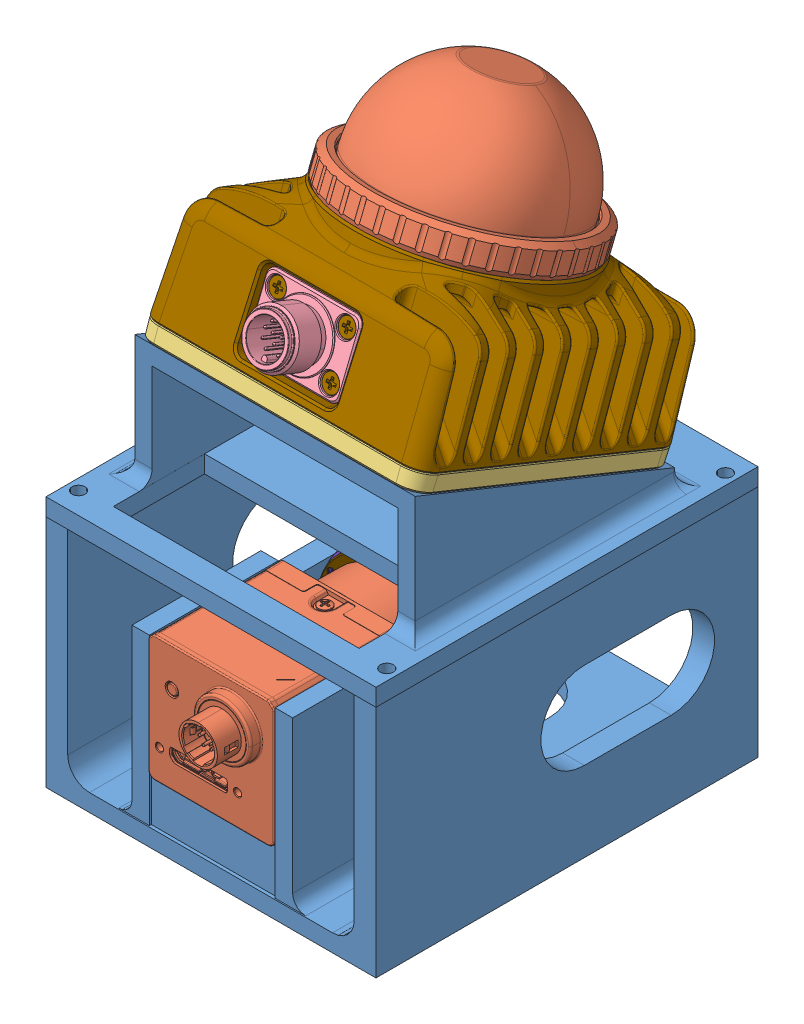
SolidWorks assembly A_LIV_Eye, configuration 默认. Lengths in mm.
Overall size (76 144.66 105.02).
33 component instances, 27 part files, 14 mates.
Components (placement in the parent):
- camera_raw-1: camera_raw [默认] at (4.6081 3.831 102) size (76 54 88)
- MV-CU013-A0UMUC.stp-1: MV-CU013-A0UMUC.stp [默认] at (4.6081 3.831 102) size (29.05 29.28 51.22)
- MVL-HF0628M-6MPE.stp-1: MVL-HF0628M-6MPE.stp [默认] at (4.6081 3.831 59.39) x (1 0 0) z (0 1 0) size (39 50.08 42.34)
  - MVL-HF0628M-6MPE_ASM_32_1_ASM.stp-1: MVL-HF0628M-6MPE_ASM_32_1_ASM.stp [默认] at origin size (39 50.08 42.34)
    - MVL-HF0628M-6MPE-201_7_1.stp-1: MVL-HF0628M-6MPE-201_7_1.stp [默认] at origin size (39 41.16 39)
    - MVL-HF0628M-6MPE-101_6_1.stp-1: MVL-HF0628M-6MPE-101_6_1.stp [默认] at (0 -2.03 0) size (36.7 28.22 36.7)
    - MVL-HF0628M-6MPE-301_6_1.stp-1: MVL-HF0628M-6MPE-301_6_1.stp [默认] at (0 -12.66 0) size (31.8 9 31.8)
    - MVL-HF0628M-6MPE-308_9_1.stp-1: MVL-HF0628M-6MPE-308_9_1.stp [默认] at (0 -11.96 0) size (31.82 2.5 31.82)
    - MVL-HF0628M-6MPE-202_4_1.stp-1: MVL-HF0628M-6MPE-202_4_1.stp [默认] at (0 -18.56 0) size (31.8 12.5 31.8)
    - MVL-HF0628M-6MPE403_6_1.stp-1: MVL-HF0628M-6MPE403_6_1.stp [默认] at (0 -21.66 0) size (33 9.2 33)
    - MVL-HF0628M-6MPE-401_4_1.stp-1: MVL-HF0628M-6MPE-401_4_1.stp [默认] at (0 -23.36 0) size (22.1 17.8 22.1)
    - MVL-HF0628M-6MPE-109_16_1.stp-1: MVL-HF0628M-6MPE-109_16_1.stp [默认] at (0 -33.65 0) size (16.5 6.81 16.5)
    - MVL-HF0628M-6MPE-G1_2_1.stp-1: MVL-HF0628M-6MPE-G1_2_1.stp [默认] at (0 -0.9326 0) size (27 7.05 27)
    - MVL-HF0628M-6MPE-G9_2_1.stp-1: MVL-HF0628M-6MPE-G9_2_1.stp [默认] at (0 -39.11 0) size (8 1.55 8)
    - MVL-HF0628M-6MPE-102_1_1.stp-1: MVL-HF0628M-6MPE-102_1_1.stp [默认] at (0 -4.03 0) size (31 2.3 31)
    - MVL-HF0628M-6MPE-108_8_1.stp-1: MVL-HF0628M-6MPE-108_8_1.stp [默认] at (0 -40.66 0) size (16 2.8 16)
    - MVL-HF0628M-6MPE-501_2_1_2.stp-1: MVL-HF0628M-6MPE-501_2_1_2.stp [默认] at (0 -27.26 -22.8398) x (1 0 0) z (0 1 0) size (4 7.7 4)
    - MVL-HF0628M-6MPE-501_2_1_2.stp-2: MVL-HF0628M-6MPE-501_2_1_2.stp [默认] at (0 -16.56 -21.48) x (1 0 0) z (0 1 0) size (4 7.7 4)
    - MVL-HF0628M-6MPE-XM_1_1.stp-1: MVL-HF0628M-6MPE-XM_1_1.stp [默认] at origin size (8 0.02 8)
    - MVL-HF0628M-6MPE-502_6_1_2.stp-1: MVL-HF0628M-6MPE-502_6_1_2.stp [默认] at (12.211 -32.384 7.05) x (-1 0 0) z (0 0 1) size (2.2 4 2.2)
    - MVL-HF0628M-6MPE-502_6_1_2.stp-2: MVL-HF0628M-6MPE-502_6_1_2.stp [默认] at (0 -32.384 -14.1) x (-1 0 0) z (0 0 1) size (2.2 4 2.2)
    - MVL-HF0628M-6MPE-502_6_1_2.stp-3: MVL-HF0628M-6MPE-502_6_1_2.stp [默认] at (-12.211 -32.384 7.05) x (-1 0 0) z (0 0 1) size (2.2 4 2.2)
    - MVL-HF0628M-6MPE-203_23_1_2.stp-1: MVL-HF0628M-6MPE-203_23_1_2.stp [默认] at (0 -29.86 0) size (31.7 9.97 31.7)
- mid_raw-1: mid_raw [默认] at (4.6251 49.2753 87.5332) x (0 -0.374635 -0.927172) z (0 -0.927172 0.374635) size (83.09 76 36.68)
- mid-360-asm.stp-1: mid-360-asm.stp [默认] at (4.6251 73.3049 77.8237) x (0 0.374635 0.927172) z (-1 0 0) size (72.74 60.14 66.87)
  - MID-360_4_1.stp-1: MID-360_4_1.stp [默认] at origin size (51.01 27.17 51.01)
  - MID-360_4_2.stp-1: MID-360_4_2.stp [默认] at origin size (64.79 8.1 64.79)
  - MID-360_4_3.stp-1: MID-360_4_3.stp [默认] at origin size (13.8 16 22)
  - MID-360_4_4.stp-1: MID-360_4_4.stp [默认] at origin size (0.41 0.09 0.09)
  - MID-360_4_5.stp-1: MID-360_4_5.stp [默认] at origin size (0.41 0.09 0.09)
  - MID-360_4_6.stp-1: MID-360_4_6.stp [默认] at origin size (0.41 0.09 0.09)
  - MID-360_4_7.stp-1: MID-360_4_7.stp [默认] at origin size (0.41 0.09 0.09)
  - MID-360_4_ASM.stp-1: MID-360_4_ASM.stp [默认] at origin size (71.75 36.34 66.87)
Mates (geometry in assembly coordinates):
- 同心1: concentric anti-aligned: cylinder of camera_raw-1 through (4.6081 -25.569 127.8) axis (0 1 0) radius 1.55; cylinder of MV-CU013-A0UMUC.stp-1 through (4.6081 -7.6148 127.8) axis (0 -1 0) radius 1.25
- 重合1: coincident anti-aligned: plane of camera_raw-1 through (4.6081 -10.569 102) normal (0 1 0); plane of MV-CU013-A0UMUC.stp-1 through (4.6081 -10.569 117.5) normal (0 -1 0)
- 重合2: coincident anti-aligned: plane of MV-CU013-A0UMUC.stp-1 through (4.6081 3.831 100.55) normal (0 0 -1); plane of MVL-HF0628M-6MPE.stp-1/MVL-HF0628M-6MPE_ASM_32_1_ASM.stp-1/MVL-HF0628M-6MPE-108_8_1.stp-1 through (4.6081 3.831 100.55) normal (0 0 1)
- 同心3: concentric anti-aligned: cylinder of MV-CU013-A0UMUC.stp-1 through (4.6081 3.831 103.9992) axis (0 0 -1) radius 12.35; cylinder of MVL-HF0628M-6MPE.stp-1/MVL-HF0628M-6MPE_ASM_32_1_ASM.stp-1/MVL-HF0628M-6MPE-203_23_1_2.stp-1 through (4.6081 3.831 88.7513) axis (0 0 1) radius 12.1
- 重合3: coincident anti-aligned: plane of camera_raw-1 through (4.6081 29.431 102) normal (0 1 0); plane of mid_raw-1 through (4.6251 29.431 87.5332) normal (0 -1 0)
- 同心6: concentric aligned: cylinder of camera_raw-1 through (-30.8919 21.431 49) axis (0 1 0) radius 1.4; circle of mid_raw-1
- 同心7: concentric aligned: cylinder of camera_raw-1 through (40.1081 21.431 49) axis (0 1 0) radius 1.4; cylinder of mid_raw-1 through (40.1081 -31.269 49) axis (0 1 0) radius 1.5
- 同心8: concentric anti-aligned: cylinder of mid_raw-1 through (-13.3749 36.5754 66.7796) axis (0 0.927172 -0.374635) radius 1.5; cylinder of mid-360-asm.stp-1/MID-360_4_2.stp-1 through (-13.3749 45.0089 63.3719) axis (0 -0.927172 0.374635) radius 1.25
- 同心9: concentric anti-aligned: cylinder of mid_raw-1 through (22.6251 54.5578 111.2839) axis (0 0.927172 -0.374635) radius 1.5; cylinder of mid-360-asm.stp-1/MID-360_4_2.stp-1 through (22.6251 62.9914 107.8762) axis (0 -0.927172 0.374635) radius 1.25
- 重合4: coincident anti-aligned: plane of mid_raw-1 through (4.6251 49.2753 87.5332) normal (0 0.927172 -0.374635); plane of mid-360-asm.stp-1/MID-360_4_2.stp-1 through (4.6251 49.2753 87.5332) normal (0 -0.927172 0.374635)
- 同心10: concentric aligned: cylinder of camera_raw-1 through (40.1081 19.431 127) axis (0 1 0) radius 1.5; cylinder of mid_raw-1 through (40.1081 -31.269 127) axis (0 1 0) radius 1.5
- 同心11: concentric aligned: cylinder of camera_raw-1 through (4.6081 -9.569 127.8) axis (0 -1 0) radius 1.6; cylinder of MV-CU013-A0UMUC.stp-1 through (4.6081 -7.6148 127.8) axis (0 -1 0) radius 1.25
- 同心12: concentric aligned: cylinder of camera_raw-1 through (-30.8919 19.431 49) axis (0 1 0) radius 1.5; cylinder of mid_raw-1 through (-30.8919 -31.269 49) axis (0 1 0) radius 1.5
- 同心13: concentric aligned: cylinder of camera_raw-1 through (40.1081 19.431 49) axis (0 1 0) radius 1.5; cylinder of mid_raw-1 through (40.1081 -31.269 49) axis (0 1 0) radius 1.5
